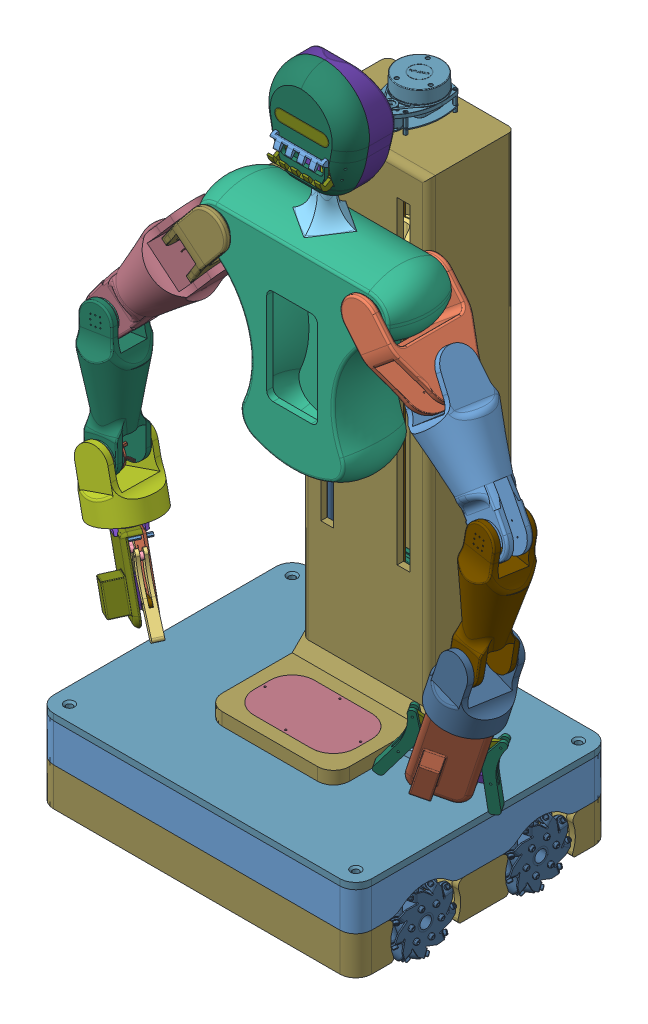
SolidWorks assembly total assembly of jaloul, configuration Défaut. Lengths in mm. (continued)
Components (placement in the parent): (continued)
- assemblt jaloul main two-1: assemblt jaloul main two [Défaut] at (-8.2808 774.6085 403.5033) x (0.999385 -0.035073 0) z (0 0 1) size (752.19 900.92 286) (continued)
  - assembly gripper  jalloul-1: assembly gripper  jalloul [Défaut] at (-235.5373 -657.7977 251.6936) x (0.796305 0.294379 0.528431) z (0.51977 0.113862 -0.846685) size (200.08 125.27 59) (continued)
    - yed jaloul-2: yed jaloul [Défaut] at (-33.5355 -10.2294 125.7) x (-0.933099 -0.359619 0) z (0 0 -1) size (39.43 112.05 15.1)
    - guidage YED JALLOUL-2: guidage YED JALLOUL [Défaut] at (-32.5775 -28.3808 115.7) x (0.926239 0.376938 0) z (0 0 1) size (50 10 5)
  - body of the robot-1: body of the robot [Défaut] at (52.9043 -73.7572 144.4967) x (0.999385 0.035073 0) z (0 0 1) size (328.01 328.01 100)
  - link 4-1: link 4 [Défaut] at (-225.981 -552.3767 191.2696) x (-0.067124 -0.087188 -0.993928) z (0.948555 0.303351 -0.09067) size (98.62 100 98.62)
  - 4015 Motor.STEP-7: 4015 Motor.STEP [Défaut] at (-201.7163 -558.9362 147.4466) x (-0.127352 -0.106316 -0.986143) z (-0.942361 -0.297187 0.153738) size (63.54 36.6 63.54)
    - 4015定子.STEP-1: 4015定子.STEP [Défaut] at origin size (45.94 27.09 45.92)
    - MISUMI_C-E6800ZZ.STEP-1: MISUMI_C-E6800ZZ.STEP [Défaut] at (0 21.6 0) x (0 -1 0) z (-0.009932 0 0.999951) size (5 19 19)
    - MISUMI_C-E6800ZZ.STEP-2: MISUMI_C-E6800ZZ.STEP [Défaut] at (0 8 0) x (0 -1 0) z (-0.587995 0 0.808864) size (5 19 19)
    - 转子铝盖.STEP-1: 转子铝盖.STEP [Défaut] at (0 24 0) x (-0.665718 0 -0.746203) z (-0.746203 0 0.665718) size (45 23.5 45)
    - 磁钢片.STEP-1: 磁钢片.STEP [Défaut] at (5.7872 12.75 -20.8182) x (0.963466 0 0.267832) z (-0.267832 0 0.963466) size (4 16.5 1.3)
    - 中间不锈钢圈.STEP-1: 中间不锈钢圈.STEP [Défaut] at (0 4.5 0) x (0.999998 0 0.002002) z (0 1 0) size (45 45 16.5)
    - 磁钢片.STEP-2: 磁钢片.STEP [Défaut] at (-0.3124 12.75 -21.6054) x (0.999895 0 -0.014457) z (0.014457 0 0.999895) size (4 16.5 1.3)
    - 磁钢片.STEP-3: 磁钢片.STEP [Défaut] at (-6.3867 12.75 -20.6422) x (0.95532 0 -0.295574) z (0.295574 0 0.95532) size (4 16.5 1.3)
    - 磁钢片.STEP-4: 磁钢片.STEP [Défaut] at (-11.9435 12.75 -18.0067) x (0.83335 0 -0.552746) z (0.552746 0 0.83335) size (4 16.5 1.3)
    - 磁钢片.STEP-5: 磁钢片.STEP [Défaut] at (-16.5328 12.75 -13.9124) x (0.643867 0 -0.765138) z (0.765138 0 0.643867) size (4 16.5 1.3)
    - 磁钢片.STEP-6: 磁钢片.STEP [Défaut] at (-19.7827 12.75 -8.6911) x (0.402221 0 -0.915542) z (0.915542 0 0.402221) size (4 16.5 1.3)
    - 磁钢片.STEP-7: 磁钢片.STEP [Défaut] at (-21.4299 12.75 -2.7656) x (0.12799 0 -0.991775) z (0.991775 0 0.12799) size (4 16.5 1.3)
    - 磁钢片.STEP-8: 磁钢片.STEP [Défaut] at (-21.341 12.75 3.384) x (-0.15661 0 -0.987661) z (0.987661 0 -0.15661) size (4 16.5 1.3)
    - 磁钢片.STEP-9: 磁钢片.STEP [Défaut] at (-19.5232 12.75 9.2593) x (-0.428522 0 -0.903531) z (0.903531 0 -0.428522) size (4 16.5 1.3)
    - 磁钢片.STEP-10: 磁钢片.STEP [Défaut] at (-16.1237 12.75 14.3846) x (-0.665718 0 -0.746203) z (0.746203 0 -0.665718) size (4 16.5 1.3)
    - 磁钢片.STEP-11: 磁钢片.STEP [Défaut] at (-11.418 12.75 18.3445) x (-0.848982 0 -0.528423) z (0.528423 0 -0.848982) size (4 16.5 1.3)
    - 磁钢片.STEP-12: 磁钢片.STEP [Défaut] at (-5.7872 12.75 20.8182) x (-0.963466 0 -0.267832) z (0.267832 0 -0.963466) size (4 16.5 1.3)
    - 磁钢片.STEP-13: 磁钢片.STEP [Défaut] at (0.3124 12.75 21.6054) x (-0.999895 0 0.014457) z (-0.014457 0 -0.999895) size (4 16.5 1.3)
    - 磁钢片.STEP-14: 磁钢片.STEP [Défaut] at (6.3867 12.75 20.6422) x (-0.95532 0 0.295574) z (-0.295574 0 -0.95532) size (4 16.5 1.3)
    - 磁钢片.STEP-15: 磁钢片.STEP [Défaut] at (11.9435 12.75 18.0067) x (-0.83335 0 0.552746) z (-0.552746 0 -0.83335) size (4 16.5 1.3)
    - 磁钢片.STEP-16: 磁钢片.STEP [Défaut] at (16.5328 12.75 13.9124) x (-0.643867 0 0.765138) z (-0.765138 0 -0.643867) size (4 16.5 1.3)
    - 磁钢片.STEP-17: 磁钢片.STEP [Défaut] at (19.7827 12.75 8.6911) x (-0.402221 0 0.915542) z (-0.915542 0 -0.402221) size (4 16.5 1.3)
    - 磁钢片.STEP-18: 磁钢片.STEP [Défaut] at (21.4299 12.75 2.7656) x (-0.12799 0 0.991775) z (-0.991775 0 -0.12799) size (4 16.5 1.3)
    - 磁钢片.STEP-19: 磁钢片.STEP [Défaut] at (21.341 12.75 -3.384) x (0.15661 0 0.987661) z (-0.987661 0 0.15661) size (4 16.5 1.3)
    - 磁钢片.STEP-20: 磁钢片.STEP [Défaut] at (19.5232 12.75 -9.2593) x (0.428522 0 0.903531) z (-0.903531 0 0.428522) size (4 16.5 1.3)
    - 磁钢片.STEP-21: 磁钢片.STEP [Défaut] at (16.1237 12.75 -14.3846) x (0.665718 0 0.746203) z (-0.746203 0 0.665718) size (4 16.5 1.3)
    - 磁钢片.STEP-22: 磁钢片.STEP [Défaut] at (11.418 12.75 -18.3445) x (0.848982 0 0.528423) z (-0.528423 0 0.848982) size (4 16.5 1.3)
    - 径向磁环.STEP-1: 径向磁环.STEP [Défaut] at (0 0.5 0) x (0.972164 0 0.234302) z (0 -1 0) size (10 10 2.5)
    - 径向磁环固定环.STEP-1: 径向磁环固定环.STEP [Défaut] at (0 -2 0) x (0.933781 0 0.357846) z (0 1 0) size (11.2 12.93 5)
    - 铜柱M2.5x4+4.STEP-1: 铜柱M2.5x4+4.STEP [Défaut] at (14 -4 0) size (5 8 5.77)
    - 铜柱M2.5x4+4.STEP-2: 铜柱M2.5x4+4.STEP [Défaut] at (0 -4 -14) x (0.982082 0 -0.188455) z (0.188455 0 0.982082) size (5 8 5.77)
    - 铜柱M2.5x4+4.STEP-3: 铜柱M2.5x4+4.STEP [Défaut] at (0 -4 14) x (0.918365 0 -0.395734) z (0.395734 0 0.918365) size (5 8 5.77)
    - 铜柱M2.5x4+4.STEP-4: 铜柱M2.5x4+4.STEP [Défaut] at (-14 -4 0) x (0.8 0 -0.6) z (0.6 0 0.8) size (5 8 5.77)
    - AS5600磁编码器-圆.STEP-1: AS5600磁编码器-圆.STEP [Défaut] at (-0.3592 -5.6 0) x (0.707107 0 -0.707107) z (0 1 0) size (31.97 31.97 7.67)
    - 铜柱M2.5x7+4.STEP-1: 铜柱M2.5x7+4.STEP [Défaut] at (0 -12.6 -14) x (0.898383 0 -0.439214) z (0.439214 0 0.898383) size (5 11 5.77)
    - 铜柱M2.5x7+4.STEP-2: 铜柱M2.5x7+4.STEP [Défaut] at (-14 -12.6 0) x (0.799513 0 -0.600648) z (0.600648 0 0.799513) size (5 11 5.77)
    - 铜柱M2.5x7+4.STEP-3: 铜柱M2.5x7+4.STEP [Défaut] at (14 -12.6 0) x (0.651231 0 -0.758879) z (0.758879 0 0.651231) size (5 11 5.77)
    - 铜柱M2.5x7+4.STEP-4: 铜柱M2.5x7+4.STEP [Défaut] at (0 -12.6 14) x (0.455178 0 -0.890401) z (0.890401 0 0.455178) size (5 11 5.77)
  - dawera grippaa hehe-1: dawera grippaa hehe [Défaut] at (-194.2904 -581.7093 148.9428) x (0.796305 0.294379 0.528431) z (0.309414 -0.948882 0.062341) size (50 50 15)
  - Symétriedawera grippaa hehe-2: Symétriedawera grippaa hehe [Défaut] at (335.0996 -563.1307 148.9428) x (-0.814983 0.237831 0.528431) z (0.242134 0.968238 -0.062341) size (50 50 15)
  - Symétrielink 4-2: Symétrielink 4 [Défaut] at (364.6559 -531.6486 191.2696) x (0.073071 -0.082268 -0.993928) z (0.967487 -0.236108 0.09067) size (98.62 100 98.62)
  - Symétrieassembly gripper  jalloul-3: Symétrieassembly gripper  jalloul [Défaut] at (381.579 -636.1403 251.6936) x (-0.814983 0.237831 0.528431) z (0.526473 -0.077144 0.846685) size (200.08 125.27 68.3)
    - SymétrieBASE GRIPPER JALLOUL-1: SymétrieBASE GRIPPER JALLOUL [Défaut] at (0.9473 -0.842 -100) size (80.77 119.68 54)
    - Symétrieservo Assem-1: Symétrieservo Assem [Défaut] at (59.4312 -11.8514 -114.1715) x (-1 0 0) z (0 -1 0) size (20 45 54)
      - Symétrieservo strong junk 2-1: Symétrieservo strong junk 2 [Default] at (33.4839 -39.4715 -49.0094) size (20 45 54)
    - Symétriepignon jlayla-1: Symétriepignon jlayla [ISO - Spur gear 2.25M 14T 20PA 5FW ---S14A75H50L5.0N] at (15.9473 27.158 -120.7) x (0 0 1) z (0.171995 0.985098 0) size (5 63.26 36)
    - Symétrieentretoise gripper JALLOUL-1: Symétrieentretoise gripper JALLOUL [Défaut] at (20.9473 -45.842 -105) x (0.938027 -0.346563 0) z (0 0 1) size (5.07 5.86 35)
    - Symétrieentretoise gripper JALLOUL-2: Symétrieentretoise gripper JALLOUL [Défaut] at (-19.0527 -45.842 -104.8272) x (0.101066 -0.99488 0) z (0 0 1) size (5.07 5.86 35)
    - Symétriegripper jaloul partie inférieur chg2-1: Symétriegripper jaloul partie inférieur chg2 [Défaut] at (0.9473 -0.842 -125.7) size (80.01 120 5.01)
    - Symétrieyed jaloul-1: Symétrieyed jaloul [Défaut] at (35.4301 -10.2294 -110.7) x (0.933099 -0.359619 0) z (0 0 1) size (39.43 112.05 15.1)
    - Symétrieguidage YED JALLOUL-1: Symétrieguidage YED JALLOUL [Défaut] at (34.4721 -28.3808 -115.7) x (0.926239 -0.376938 0) z (0 0 1) size (50 10 5)
    - SymétrieSymétriepignon jlayla-1: SymétrieSymétriepignon jlayla [ISO - Spur gear 2.25M 14T 20PA 5FW ---S14A75H50L5.0N] at (-14.0527 27.158 -120.7) x (0 0 1) z (0.171995 -0.985098 0) size (5 63.26 36)
    - Symétrieyed jaloul-2: Symétrieyed jaloul [Défaut] at (-33.5355 -10.2294 -125.7) x (-0.933099 -0.359619 0) z (0 0 -1) size (39.43 112.05 15.1)
    - Symétrieguidage YED JALLOUL-2: Symétrieguidage YED JALLOUL [Défaut] at (-32.5775 -28.3808 -115.7) x (0.926239 0.376938 0) z (0 0 1) size (50 10 5)
  - SymétrieLINK 3 JALOUL-3: SymétrieLINK 3 JALOUL [Défaut] at (384.5727 -365.0326 168.8818) x (0.063286 0.994966 -0.077701) z (0.995317 -0.057224 0.077909) size (224.5 90.56 90.03)
  - Symétrielink 2 JALOUL-3: Symétrielink 2 JALOUL [Défaut] at (309.1195 -184.0258 82.9556) x (-0.660045 0.743124 -0.110033) z (0.073071 -0.082268 -0.993928) size (247.23 121.75 118.52)
  - Symétrielink 1 JALOUL-3: Symétrielink 1 JALOUL [Défaut] at (183.0137 -109.8103 159.4967) x (-0.664077 0.747664 0) z (0 0 -1) size (167.5 60.6 125)
  - sac de guidage JALOUL EL KABRAN-1: sac de guidage JALOUL EL KABRAN [Défaut] at (-9.0397 -161.9779 54.4967) x (0.999385 0.035073 0) z (-0.035073 0.999385 0) size (197.71 92.13 60)
- NEMA_235628-6.35_s.STEP-1: NEMA_235628-6.35_s.STEP [Défaut] at (54.2045 -2.1397 406.7435) x (0 -1 0) z (0 0 1) size (82 61.91 56.65)
  - Nema2356_top.STEP-1: Nema2356_top.STEP [Défaut] at (-25.5081 -82.6274 143.9932) size (12.4 56.42 56.42)
  - Nema2356_middle.STEP-1: Nema2356_middle.STEP [Défaut] at (-14.7081 17.769 14.044) size (32.8 56.4 56.4)
  - Nema2356_bottom.STEP-1: Nema2356_bottom.STEP [Défaut] at (18.0919 -112.7781 -165.2225) size (11 56.4 56.4)
  - Nema2356_axis.STEP-1: Nema2356_axis.STEP [Défaut] at (-52.9081 -12.2004 -20.8718) x (1 0 0) z (0 -0.367241 0.930126) size (78 6.35 6.35)
  - Nema2356_gultnis.STEP-1: Nema2356_gultnis.STEP [Défaut] at (-25.7081 -12.2004 -20.8718) x (1 0 0) z (0 0.415119 0.909767) size (3 11.6 11.6)
  - Nema2356_gultnis.STEP-2: Nema2356_gultnis.STEP [Défaut] at (22.0919 -12.2004 -20.8718) size (3 11.6 11.6)
  - Nema2356_screv.STEP-1: Nema2356_screv.STEP [Défaut] at (-13.1349 -28.2433 4.9528) size (54.01 5 5)
  - Nema2356_screv.STEP-2: Nema2356_screv.STEP [Défaut] at (-13.1349 3.8425 4.9528) size (54.01 5 5)
  - Nema2356_screv.STEP-3: Nema2356_screv.STEP [Défaut] at (-13.1349 -28.2433 -46.6964) size (54.01 5 5)
  - Nema2356_screv.STEP-4: Nema2356_screv.STEP [Défaut] at (-13.1349 3.8425 -46.6964) size (54.01 5 5)
  - Nema2356_contact.STEP-1: Nema2356_contact.STEP [Défaut] at (21.7519 15.9996 -20.8718) size (7.63 5.5 30.97)
- NEMA17_Coupler-1: NEMA17_Coupler [Default] at (42.0041 37.7684 385.8717) x (0.951848 0 -0.306569) z (0.306569 0 0.951848) size (20 26 20)
- entretoise fixation steeper nema A 23 système de translation-1: entretoise fixation steeper nema A 23 système de translation [Défaut] at (18.3298 -31.2316 362.1974) x (-0.440874 0 0.897569) z (0 1 0) size (6.06 7 49)
- entretoise fixation steeper nema A 23 système de translation-3: entretoise fixation steeper nema A 23 système de translation [Défaut] at (65.6784 -31.2316 362.1974) x (1 0 0) z (0 1 0) size (6.06 7 49)
- entretoise fixation steeper nema A 23 système de translation-4: entretoise fixation steeper nema A 23 système de translation [Défaut] at (18.3298 -31.2316 409.5461) x (-0.393751 0 -0.919217) z (0 1 0) size (6.06 7 49)
- entretoise fixation steeper nema A 23 système de translation-5: entretoise fixation steeper nema A 23 système de translation [Défaut] at (65.6784 -31.2316 409.5461) x (0.722733 0 -0.691128) z (0 1 0) size (6.06 7 49)
- angle backet 25 25 jaloul hehe-1: angle backet 25 25 jaloul hehe [Default] at (132.0041 167.3641 343) x (0 0 1) z (0 -1 0) size (17 21 21)
- LeadScrew Nut 8mm x 2mmPitch-1: LeadScrew Nut 8mm x 2mmPitch [Default] at (42.0041 649.0473 385.8717) x (-0.784692 0 -0.619886) z (0 1 0) size (22 22 16.05)
- LMH8UU-1: LMH8UU [Default] at (-41.8518 650.5473 413.3388) x (-0.866025 0 -0.5) z (-0.5 0 0.866025) size (20 23 32)
- LMH8UU-2: LMH8UU [Default] at (125.86 650.5473 413.3388) x (-0.866025 0 0.5) z (0.5 0 0.866025) size (20 23 32)
- tige fileté provisoire pour fileté-1: tige fileté provisoire pour fileté [Défaut] at (42.0041 750.7684 385.8717) x (1 0 0) z (0 -1 0) size (8 8 700)
- tige lisse guidage M8 L 722-1: tige lisse guidage M8 L 722 [Défaut] at (-41.8518 750.7684 413.3388) x (0.400649 0 0.916232) z (0 -1 0) size (8 8 722)
- tige lisse guidage M8 L 722-2: tige lisse guidage M8 L 722 [Défaut] at (125.86 750.7684 413.3388) x (0.400649 0 0.916232) z (0 -1 0) size (8 8 722)
- pièce de fixation-1: pièce de fixation [Défaut] at (125.86 38.7684 413.3388) x (-0.953717 0 -0.300706) z (0 -1 0) size (25.26 55.08 12.09)
- pièce de fixation-2: pièce de fixation [Défaut] at (-41.8518 38.7684 413.3388) x (0.953717 0 -0.300706) z (0 -1 0) size (25.26 55.08 12.09)
- cache système translation jaloul-1: cache système translation jaloul [Défaut] at (42.0041 28.7684 375.5) x (1 0 0) z (0 1 0) size (200 285 757)
- séparation en plexiglasse et porteur de charge-1: séparation en plexiglasse et porteur de charge [Défaut] at (40.896 43.7684 525.0845) x (1 0 0) z (0 1 0) size (160 95 5)
- RP-Lidar-1: RP-Lidar [Default] at (174.9217 66.0761 448.5533) x (0 0 1) z (-1 0 0) size (99.56 53.5 71.78)
- pièce de fixation-3: pièce de fixation [Défaut] at (-41.8518 740.7684 413.3388) x (-0.953717 0 0.300706) z (0 1 0) size (25.26 55.08 12.09)
- pièce de fixation-4: pièce de fixation [Défaut] at (125.86 740.7684 413.3388) x (0.953717 0 0.300706) z (0 1 0) size (25.26 55.08 12.09)
- prfoilé aliminuim liason entre les murs cache sys trs-1: prfoilé aliminuim liason entre les murs cache sys trs [Défaut] at (-187.9959 157.3641 353) x (0 0 1) z (-1 0 0) size (20 20 180)
- angle backet 25 25 jaloul hehe-2: angle backet 25 25 jaloul hehe [Default] at (-47.9959 167.3641 360) x (0 0 -1) z (0 -1 0) size (17 21 21)
- angle backet 25 25 jaloul hehe-32: angle backet 25 25 jaloul hehe [Default] at (132.0041 442.3641 343) x (0 0 1) z (0 -1 0) size (17 21 21)
- angle backet 25 25 jaloul hehe-33: angle backet 25 25 jaloul hehe [Default] at (132.0041 717.3641 343) x (0 0 1) z (0 -1 0) size (17 21 21)
- prfoilé aliminuim liason entre les murs cache sys trs-7: prfoilé aliminuim liason entre les murs cache sys trs [Défaut] at (-187.9959 432.3641 353) x (0 0 1) z (-1 0 0) size (20 20 180)
- prfoilé aliminuim liason entre les murs cache sys trs-8: prfoilé aliminuim liason entre les murs cache sys trs [Défaut] at (-187.9959 707.3641 353) x (0 0 1) z (-1 0 0) size (20 20 180)
- angle backet 25 25 jaloul hehe-34: angle backet 25 25 jaloul hehe [Default] at (-47.9959 442.3641 360) x (0 0 -1) z (0 -1 0) size (17 21 21)
- angle backet 25 25 jaloul hehe-35: angle backet 25 25 jaloul hehe [Default] at (-47.9959 717.3641 360) x (0 0 -1) z (0 -1 0) size (17 21 21)
Mates (geometry in assembly coordinates):
- Coïncidente6: coincident anti-aligned: plane of assembly bas robot jlayla-1/BASE ROBOT JALOUL-1 through (42.0041 -31.2316 508) normal (0 1 0); plane of NEMA_235628-6.35_s.STEP-1/Nema2356_bottom.STEP-1 through (58.9141 -31.2316 412.0717) normal (0 -1 0)
- Coaxiale1: concentric anti-aligned: cylinder of NEMA_235628-6.35_s.STEP-1/Nema2356_axis.STEP-1 through (42.0041 -27.2316 385.8717) axis (0 1 0) radius 3.175; cylinder of NEMA17_Coupler-1 through (42.0041 37.7684 385.8717) axis (0 -1 0) radius 10
- Distance4: distance = 13 mm anti-aligned: plane of NEMA17_Coupler-1 through (44.6407 37.7684 385.0225) normal (0 -1 0); plane of NEMA_235628-6.35_s.STEP-1/Nema2356_axis.STEP-1 through (42.0041 50.7684 385.8717) normal (0 1 0)
- Coïncidente8: coincident anti-aligned: plane of assembly bas robot jlayla-1/BASE ROBOT JALOUL-1 through (42.0041 -31.2316 508) normal (0 1 0); plane of entretoise fixation steeper nema A 23 système de translation-1 through (18.3298 -31.2316 362.1974) normal (0 -1 0)
- Coaxiale2: concentric anti-aligned: cylinder of NEMA_235628-6.35_s.STEP-1/Nema2356_top.STEP-1 through (18.3298 18.5684 362.1974) axis (0 1 0) radius 2; cylinder of entretoise fixation steeper nema A 23 système de translation-1 through (18.3298 17.7684 362.1974) axis (0 -1 0) radius 2
- Coïncidente11: coincident anti-aligned: plane of assembly bas robot jlayla-1/BASE ROBOT JALOUL-1 through (42.0041 -31.2316 508) normal (0 1 0); plane of entretoise fixation steeper nema A 23 système de translation-3 through (65.6784 -31.2316 362.1974) normal (0 -1 0)
- Coaxiale3: concentric anti-aligned: cylinder of NEMA_235628-6.35_s.STEP-1/Nema2356_top.STEP-1 through (65.6784 18.5684 362.1974) axis (0 1 0) radius 2; axis of entretoise fixation steeper nema A 23 système de translation-3 through (65.6784 17.7684 362.1974) axis (0 -1 0)
- Coaxiale4: concentric anti-aligned: cylinder of NEMA_235628-6.35_s.STEP-1/Nema2356_top.STEP-1 through (65.6784 18.5684 409.5461) axis (0 1 0) radius 2; cylinder of entretoise fixation steeper nema A 23 système de translation-5 through (65.6784 17.7684 409.5461) axis (0 -1 0) radius 2
- Coïncidente12: coincident anti-aligned: plane of assembly bas robot jlayla-1/BASE ROBOT JALOUL-1 through (42.0041 -31.2316 508) normal (0 1 0); plane of entretoise fixation steeper nema A 23 système de translation-5 through (65.6784 -31.2316 409.5461) normal (0 -1 0)
- Coaxiale5: concentric anti-aligned: cylinder of NEMA_235628-6.35_s.STEP-1/Nema2356_top.STEP-1 through (18.3298 18.5684 409.5461) axis (0 1 0) radius 2; cylinder of entretoise fixation steeper nema A 23 système de translation-4 through (18.3298 17.7684 409.5461) axis (0 -1 0) radius 2
- Coaxiale6: concentric aligned: cylinder of assemblt jaloul main two-1/sac de guidage JALOUL EL KABRAN-1 through (42.0041 640.5473 385.8717) axis (0 1 0) radius 5.25; cylinder of LeadScrew Nut 8mm x 2mmPitch-1 through (42.0041 645.5473 385.8717) axis (0 1 0) radius 11
- Coïncidente14: coincident anti-aligned: plane of assemblt jaloul main two-1/sac de guidage JALOUL EL KABRAN-1 through (42.0041 645.5473 385.8717) normal (0 1 0); plane of LeadScrew Nut 8mm x 2mmPitch-1 through (42.0041 645.5473 385.8717) normal (0 -1 0)
- Largeur3: width anti-aligned: plane of NEMA_235628-6.35_s.STEP-1/Nema2356_middle.STEP-1 through (13.8041 -20.2316 402.7817) normal (-1 0 0); plane of assembly bas robot jlayla-1/BASE ROBOT JALOUL-1 through (70.2041 -20.2316 368.9617) normal (1 0 0); plane of NEMA_235628-6.35_s.STEP-1/Nema2356_middle.STEP-1 through (292.0041 -31.2316 308) normal (1 0 0); plane of assembly bas robot jlayla-1/BASE ROBOT JALOUL-1 through (-207.9959 -31.2316 308) normal (-1 0 0)
- Coaxiale8: concentric anti-aligned: cylinder of NEMA17_Coupler-1 through (42.0041 37.7684 385.8717) axis (0 -1 0) radius 10; cylinder of LeadScrew Nut 8mm x 2mmPitch-1 through (42.0041 645.5473 385.8717) axis (0 1 0) radius 11
- Parallèle1: parallel aligned: plane of assembly bas robot jlayla-1/BASE ROBOT JALOUL-1 through (292.0041 -31.2316 308) normal (0 0 -1); plane of assemblt jaloul main two-1/body of the robot-1 through (162.0041 669.0412 458) normal (0 0 -1)
- Largeur4: width aligned: plane of assembly bas robot jlayla-1/BASE ROBOT JALOUL-1 through (292.0041 -31.2316 708) normal (0 0 1); plane of assemblt jaloul main two-1/body of the robot-1 through (292.0041 -31.2316 308) normal (0 0 -1); plane of assembly bas robot jlayla-1/BASE ROBOT JALOUL-1 through (162.0041 669.0412 558) normal (0 0 1); plane of assemblt jaloul main two-1/body of the robot-1 through (162.0041 669.0412 458) normal (0 0 -1)
- Coaxiale9: concentric aligned: cylinder of assemblt jaloul main two-1/sac de guidage JALOUL EL KABRAN-1 through (-41.8518 640.5473 413.3388) axis (0 1 0) radius 7.7898; cylinder of LMH8UU-1 through (-41.8518 627.5473 413.3388) axis (0 1 0) radius 7.5
- Parallèle2: parallel aligned: plane of assemblt jaloul main two-1/sac de guidage JALOUL EL KABRAN-1 through (2.0041 673.0473 397.3782) normal (-0.866025 0 -0.5); plane of LMH8UU-1 through (-44.267 645.5473 397.5222) normal (-0.866025 0 -0.5)
- Coïncidente19: coincident anti-aligned: plane of assemblt jaloul main two-1/sac de guidage JALOUL EL KABRAN-1 through (-41.8518 645.5473 413.3388) normal (0 1 0); plane of LMH8UU-1 through (-41.8518 645.5473 413.3388) normal (0 -1 0)
- Coaxiale10: concentric aligned: circle of assemblt jaloul main two-1/sac de guidage JALOUL EL KABRAN-1; cylinder of LMH8UU-2 through (125.86 627.5473 413.3388) axis (0 1 0) radius 7.5
- Parallèle3: parallel anti-aligned: plane of assemblt jaloul main two-1/sac de guidage JALOUL EL KABRAN-1 through (117.0041 673.0473 458) normal (0.866025 0 -0.5); plane of LMH8UU-2 through (110.9547 645.5473 407.5222) normal (-0.866025 0 0.5)
- Coïncidente21: coincident anti-aligned: plane of assemblt jaloul main two-1/sac de guidage JALOUL EL KABRAN-1 through (125.86 645.5473 413.3388) normal (0 1 0); plane of LMH8UU-2 through (125.86 645.5473 413.3388) normal (0 -1 0)
- Coïncidente22: coincident anti-aligned: plane of assembly bas robot jlayla-1/BASE ROBOT JALOUL-1 through (42.0041 -31.2316 508) normal (0 1 0); plane of entretoise fixation steeper nema A 23 système de translation-4 through (18.3298 -31.2316 409.5461) normal (0 -1 0)
- Coaxiale11: concentric anti-aligned: cylinder of NEMA17_Coupler-1 through (42.0041 37.7684 385.8717) axis (0 -1 0) radius 10; cylinder of tige fileté provisoire pour fileté-1 through (42.0041 50.7684 385.8717) axis (0 1 0) radius 4
- Distance5: distance = 13 mm anti-aligned: plane of tige fileté provisoire pour fileté-1 through (42.0041 50.7684 385.8717) normal (0 -1 0); plane of NEMA17_Coupler-1 through (51.2846 63.7684 382.8827) normal (0 1 0)
- Coaxiale12: concentric aligned: cylinder of LMH8UU-1 through (-41.8518 627.5473 413.3388) axis (0 1 0) radius 7.5; cylinder of tige lisse guidage M8 L 722-1 through (-41.8518 28.7684 413.3388) axis (0 1 0) radius 4
- Coïncidente24: coincident anti-aligned: plane of assembly bas robot jlayla-1/cache supérieur fixe jlayla-1 through (267.0041 28.7684 333) normal (0 1 0); plane of tige lisse guidage M8 L 722-1 through (-41.8518 28.7684 413.3388) normal (0 -1 0)
- Coaxiale13: concentric aligned: cylinder of LMH8UU-2 through (125.86 627.5473 413.3388) axis (0 1 0) radius 7.5; cylinder of tige lisse guidage M8 L 722-2 through (125.86 28.7684 413.3388) axis (0 1 0) radius 4
- Coïncidente25: coincident anti-aligned: plane of assembly bas robot jlayla-1/cache supérieur fixe jlayla-1 through (267.0041 28.7684 333) normal (0 1 0); circle of tige lisse guidage M8 L 722-2
- Coïncidente26: coincident anti-aligned: plane of assembly bas robot jlayla-1/cache supérieur fixe jlayla-1 through (267.0041 28.7684 333) normal (0 1 0); plane of pièce de fixation-1 through (125.86 28.7684 413.3388) normal (0 -1 0)
- Coaxiale14: concentric aligned: cylinder of tige lisse guidage M8 L 722-2 through (125.86 28.7684 413.3388) axis (0 1 0) radius 4; cylinder of pièce de fixation-1 through (125.86 28.7684 413.3388) axis (0 1 0) radius 4
- Angle1: planar angle = 2.96706 rad aligned: plane of assembly bas robot jlayla-1/cache supérieur fixe jlayla-1 through (292.0041 28.7684 683) normal (1 0 0); plane of pièce de fixation-1 through (116.0119 28.7684 411.6023) normal (-0.984808 0 -0.173648)
- Coïncidente28: coincident anti-aligned: plane of assembly bas robot jlayla-1/cache supérieur fixe jlayla-1 through (267.0041 28.7684 333) normal (0 1 0); plane of pièce de fixation-2 through (-41.8518 28.7684 413.3388) normal (0 -1 0)
- Coaxiale15: concentric aligned: cylinder of tige lisse guidage M8 L 722-1 through (-41.8518 28.7684 413.3388) axis (0 1 0) radius 4; cylinder of pièce de fixation-2 through (-41.8518 28.7684 413.3388) axis (0 1 0) radius 4
- Angle2: planar angle = 2.96706 rad aligned: plane of assembly bas robot jlayla-1/cache supérieur fixe jlayla-1 through (-207.9959 28.7684 333) normal (-1 0 0); plane of pièce de fixation-2 through (-32.0037 28.7684 411.6023) normal (0.984808 0 -0.173648)
- Coïncidente30: coincident anti-aligned: plane of assembly bas robot jlayla-1/cache supérieur fixe jlayla-1 through (267.0041 28.7684 333) normal (0 1 0); plane of cache système translation jaloul-1 through (42.0041 28.7684 375.5) normal (0 -1 0)
- Coïncidente31: coincident aligned: plane of assembly bas robot jlayla-1/BASE ROBOT JALOUL-1 through (292.0041 -31.2316 308) normal (0 0 -1); plane of cache système translation jaloul-1 through (-57.9959 755.7684 308) normal (0 0 -1)
- Largeur5: width anti-aligned: plane of assembly bas robot jlayla-1/BASE ROBOT JALOUL-1 through (292.0041 -31.2316 308) normal (1 0 0); plane of assembly bas robot jlayla-1/BASE ROBOT JALOUL-1 through (-207.9959 -31.2316 308) normal (-1 0 0); plane of cache système translation jaloul-1 through (-57.9959 755.7684 308) normal (-1 0 0); plane of cache système translation jaloul-1 through (142.0041 755.7684 308) normal (1 0 0)
- Coïncidente32: coincident anti-aligned: plane of cache système translation jaloul-1 through (87.0041 43.7684 513) normal (0 1 0); plane of séparation en plexiglasse et porteur de charge-1 through (87.0041 43.7684 513) normal (0 -1 0)
- Coaxiale16: concentric anti-aligned: cylinder of cache système translation jaloul-1 through (-2.9959 43.7684 513) axis (0 1 0) radius 35; cylinder of séparation en plexiglasse et porteur de charge-1 through (-2.9959 48.7684 513) axis (0 -1 0) radius 35
- Coïncidente33: coincident: plane of cache système translation jaloul-1 through (-37.9959 43.7684 513) normal (1 0 0); line of séparation en plexiglasse et porteur de charge-1 through (-37.9959 43.7684 513) axis (0 0 1)
- Coïncidente34: coincident anti-aligned: plane of cache système translation jaloul-1 through (42.0041 785.7684 375.5) normal (0 1 0); plane of RP-Lidar-1 through (11.4941 785.7684 327.1032) normal (0 -1 0)
- Parallèle6: parallel aligned: plane of cache système translation jaloul-1 through (-57.9959 755.7684 308) normal (-1 0 0); plane of RP-Lidar-1 through (12.4041 793.7784 368.01) normal (-1 0 0)
- Distance6: distance = 100 mm: plane of assembly; axis of RP-Lidar-1 through (42.0041 799.2548 358) axis (0 1 0); plane of cache système translation jaloul-1 through (-57.9959 755.7684 308) normal (-1 0 0)
- Distance7: distance = 50 mm: plane of assembly; axis of RP-Lidar-1 through (42.0041 799.2548 358) axis (0 1 0); plane of cache système translation jaloul-1 through (-57.9959 755.7684 308) normal (0 0 -1)
- Coaxiale17: concentric anti-aligned: cylinder of tige lisse guidage M8 L 722-1 through (-41.8518 28.7684 413.3388) axis (0 1 0) radius 4; cylinder of pièce de fixation-3 through (-41.8518 750.7684 413.3388) axis (0 -1 0) radius 4
- Coïncidente38: coincident aligned: plane of tige lisse guidage M8 L 722-1 through (-41.8518 750.7684 413.3388) normal (0 1 0); plane of pièce de fixation-3 through (-41.8518 750.7684 413.3388) normal (0 1 0)
- Coïncidente39: coincident aligned: plane of pièce de fixation-2 through (-51.6999 28.7684 415.0753) normal (-0.984808 0 0.173648); plane of pièce de fixation-3 through (-51.6999 750.7684 415.0753) normal (-0.984808 0 0.173648)
- Distance9: distance = 10 mm aligned: plane of prfoilé aliminuim liason entre les murs cache sys trs-1 through (132.0041 157.3641 353) normal (1 0 0); plane of cache système translation jaloul-1 through (142.0041 755.7684 308) normal (1 0 0)
- Coïncidente73: coincident anti-aligned: plane of angle backet 25 25 jaloul hehe-1 through (132.0041 167.3641 345) normal (0 -1 0); plane of prfoilé aliminuim liason entre les murs cache sys trs-1 through (-187.9959 167.3641 349.7) normal (0 1 0)
- Coïncidente74: coincident aligned: plane of angle backet 25 25 jaloul hehe-1 through (132.0041 167.3641 343) normal (0 0 -1); plane of prfoilé aliminuim liason entre les murs cache sys trs-1 through (-187.9959 166.3641 343) normal (0 0 -1)
- Coïncidente75: coincident aligned: plane of angle backet 25 25 jaloul hehe-1 through (132.0041 167.3641 345) normal (1 0 0); plane of prfoilé aliminuim liason entre les murs cache sys trs-1 through (132.0041 157.3641 353) normal (1 0 0)
- Distance14: distance = 35 mm aligned: plane of prfoilé aliminuim liason entre les murs cache sys trs-1 through (-187.9959 166.3641 343) normal (0 0 -1); plane of assembly bas robot jlayla-1/BASE ROBOT JALOUL-1 through (292.0041 -31.2316 308) normal (0 0 -1)
